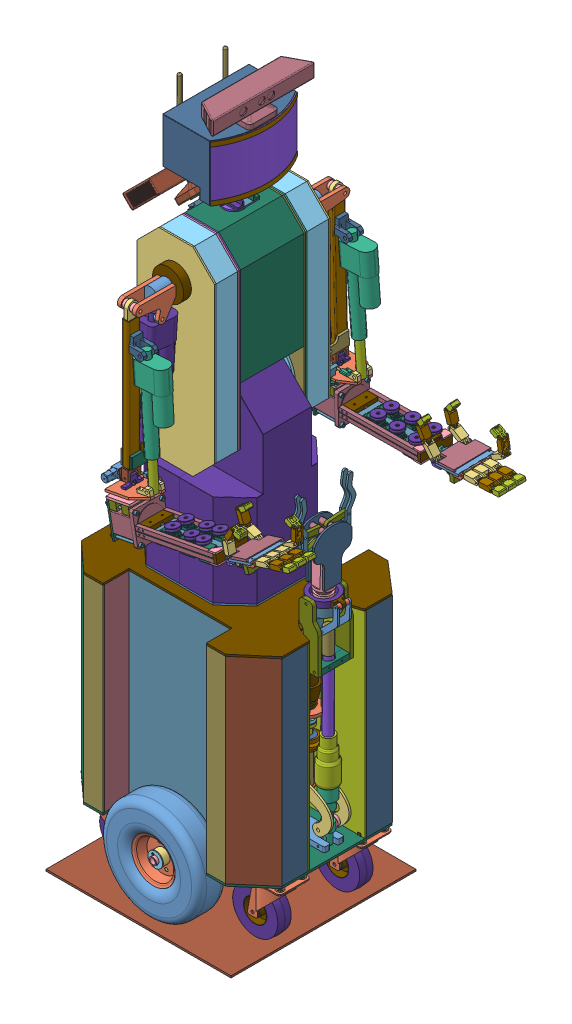
SolidWorks assembly sorbot, configuration По умолчанию. Lengths in mm. (continued)
Components (placement in the parent): (continued)
- bolt1-1: bolt1 [По умолчанию] at (252.2608 28.1179 -56.3731) x (0 0 1) z (1 0 0) size (14 40.5 16.17)
- bolt1-2: bolt1 [По умолчанию] at (172.9115 28.0264 3.3236) x (0 0 1) z (1 0 0) size (14 40.5 16.17)
- bolt1-3: bolt1 [По умолчанию] at (251.9125 28.1164 3.3175) x (0 0 1) z (1 0 0) size (14 40.5 16.17)
- bolt1-4: bolt1 [По умолчанию] at (172.9018 28.0211 -56.2899) x (0 0 1) z (1 0 0) size (14 40.5 16.17)
- bolt1-5: bolt1 [По умолчанию] at (172.7717 28.5111 -218.0055) x (0.546944 0 -0.837169) z (-0.837169 0 -0.546944) size (14 40.5 16.17)
- bolt1-6: bolt1 [По умолчанию] at (251.718 28.5111 -277.7613) x (0.546944 0 -0.837169) z (-0.837169 0 -0.546944) size (14 40.5 16.17)
- bolt1-7: bolt1 [По умолчанию] at (172.7558 28.5111 -277.7529) x (0.546944 0 -0.837169) z (-0.837169 0 -0.546944) size (14 40.5 16.17)
- bolt1-8: bolt1 [По умолчанию] at (251.8056 28.5111 -218.1439) x (0.546944 0 -0.837169) z (-0.837169 0 -0.546944) size (14 40.5 16.17)
- bolt1-9: bolt1 [По умолчанию] at (-260.5376 28.2059 -219.1987) x (0.546944 0 -0.837169) z (-0.837169 0 -0.546944) size (14 40.5 16.17)
- bolt1-10: bolt1 [По умолчанию] at (-181.6432 28.2059 -219.1307) x (0.546944 0 -0.837169) z (-0.837169 0 -0.546944) size (14 40.5 16.17)
- bolt1-11: bolt1 [По умолчанию] at (-181.4767 28.2059 -278.9161) x (0.546944 0 -0.837169) z (-0.837169 0 -0.546944) size (14 40.5 16.17)
- bolt1-12: bolt1 [По умолчанию] at (-260.5141 28.2059 -278.9485) x (0.546944 0 -0.837169) z (-0.837169 0 -0.546944) size (14 40.5 16.17)
- bolt1-13: bolt1 [По умолчанию] at (-260.8842 28.1192 -54.1025) x (-0.546944 0 0.837169) z (0.837169 0 0.546944) size (14 40.5 16.17)
- bolt1-14: bolt1 [По умолчанию] at (-181.8952 28.1192 -54.0898) x (-0.546944 0 0.837169) z (0.837169 0 0.546944) size (14 40.5 16.17)
- bolt1-15: bolt1 [По умолчанию] at (-260.8825 28.1192 5.6198) x (-0.546944 0 0.837169) z (0.837169 0 0.546944) size (14 40.5 16.17)
- bolt1-16: bolt1 [По умолчанию] at (-181.994 28.1192 5.6123) x (-0.546944 0 0.837169) z (0.837169 0 0.546944) size (14 40.5 16.17)
- bolt1.nut-1: bolt1.nut [По умолчанию] at (-181.4767 51.9368 -278.9161) x (0 0 1) z (-1 0 0) size (14 6 16.17)
- bolt1.nut-2: bolt1.nut [По умолчанию] at (-260.5141 51.9368 -278.9485) x (0 0 1) z (-1 0 0) size (14 6 16.17)
- bolt1.nut-3: bolt1.nut [По умолчанию] at (-260.5376 51.9368 -219.1987) x (0 0 1) z (-1 0 0) size (14 6 16.17)
- bolt1.nut-4: bolt1.nut [По умолчанию] at (-181.6432 51.9368 -219.1307) x (0 0 1) z (-1 0 0) size (14 6 16.17)
- bolt1.nut-5: bolt1.nut [По умолчанию] at (-181.994 51.9368 5.6123) x (0 0 -1) z (1 0 0) size (14 6 16.17)
- bolt1.nut-6: bolt1.nut [По умолчанию] at (-260.8825 51.9368 5.6198) x (0 0 -1) z (1 0 0) size (14 6 16.17)
- bolt1.nut-7: bolt1.nut [По умолчанию] at (-260.8842 51.9368 -54.1025) x (0 0 -1) z (1 0 0) size (14 6 16.17)
- bolt1.nut-8: bolt1.nut [По умолчанию] at (-181.8952 51.9368 -54.0898) x (0 0 -1) z (1 0 0) size (14 6 16.17)
- bolt1.nut-9: bolt1.nut [По умолчанию] at (172.9115 51.9368 3.3236) x (0 0 -1) z (1 0 0) size (14 6 16.17)
- bolt1.nut-10: bolt1.nut [По умолчанию] at (251.9125 51.7388 3.3175) x (0 0 -1) z (1 0 0) size (14 6 16.17)
- bolt1.nut-11: bolt1.nut [По умолчанию] at (252.2608 51.5573 -56.3731) x (0 0 -1) z (1 0 0) size (14 6 16.17)
- bolt1.nut-12: bolt1.nut [По умолчанию] at (172.9018 51.3675 -56.2899) x (0 0 -1) z (1 0 0) size (14 6 16.17)
- bolt1.nut-13: bolt1.nut [По умолчанию] at (172.7558 51.9368 -277.7529) x (0 0 1) z (-1 0 0) size (14 6 16.17)
- bolt1.nut-14: bolt1.nut [По умолчанию] at (172.7717 51.9368 -218.0055) x (0 0 1) z (-1 0 0) size (14 6 16.17)
- bolt1.nut-15: bolt1.nut [По умолчанию] at (251.718 51.9368 -277.7613) x (0 0 1) z (-1 0 0) size (14 6 16.17)
- bolt1.nut-16: bolt1.nut [По умолчанию] at (251.8056 51.9368 -218.1439) x (0 0 1) z (-1 0 0) size (14 6 16.17)
- turret.table-1: turret.table [По умолчанию] at (-20.8718 607.7934 -141.039) size (305 5 278)
- turret.center-1: turret.center [По умолчанию] at (-20.0648 607.7934 -136.9555) x (1 0 -0.000338) z (0.000338 0 1) size (90 80 90)
- body.center-1: body.center [По умолчанию] at (-20.0648 627.0246 -136.9555) size (22 355 22)
- wheel.axis.frame.fixture.p1-1: wheel.axis.frame.fixture.p1 [По умолчанию] at (40.6964 23.6368 -47.3934) x (0.999999 0 0.001149) z (-0.001149 0 0.999999) size (21.7 48.8 22.74)
- wheel.axis.frame.fixture.p1-2: wheel.axis.frame.fixture.p1 [По умолчанию] at (-54.5345 23.6368 -47.3503) size (21.7 48.8 22.74)
- wheel.axis.frame.fixture.p1-3: wheel.axis.frame.fixture.p1 [По умолчанию] at (40.6515 23.6368 -224.9519) size (21.7 48.8 22.74)
- wheel.axis.frame.fixture.p1-4: wheel.axis.frame.fixture.p1 [По умолчанию] at (-54.2945 23.6368 -224.8346) size (21.7 48.8 22.74)
- gearmotor.fixture.p2.1-1: gearmotor.fixture.p2.1 [По умолчанию] at (2.1309 53.4368 -208.1692) x (-1 0 0) z (0 0 -1) size (86 101.43 182)
- wheel.axis.frame.fixture.p2-1: wheel.axis.frame.fixture.p2 [По умолчанию] at (40.6964 51.9368 -47.3934) size (22.08 10 22.5)
- wheel.axis.frame.fixture.p2-2: wheel.axis.frame.fixture.p2 [По умолчанию] at (40.6515 53.4933 -224.9519) size (22.08 10 22.5)
- wheel.axis.frame.fixture.p2-3: wheel.axis.frame.fixture.p2 [По умолчанию] at (-54.2945 53.4933 -224.8346) size (22.08 10 22.5)
- wheel.axis.frame.fixture.p2-4: wheel.axis.frame.fixture.p2 [По умолчанию] at (-54.5345 53.4933 -47.3503) size (22.08 10 22.5)
- wall-fixture-3-2: wall-fixture-3 [По умолчанию] at (-150.6756 56.9368 4.4522) size (287.58 65 40)
- wall-fixture-3-1-1: wall-fixture-3-1 [По умолчанию] at (-154.6756 56.9368 4.4522) x (0 0 -1) z (1 0 0) size (74 65 40)
- wall-fixture-3-2-1: wall-fixture-3-2 [По умолчанию] at (-154.6756 56.9368 74.4522) size (42 65 40)
- wall-fixture-3-3-1: wall-fixture-3-3 [По умолчанию] at (-194.4824 56.9368 75.4251) x (0.73854 0 0.67421) z (-0.67421 0 0.73854) size (116.95 65 40)
- ground-1: ground [По умолчанию] at (-17.2598 -128.0632 -134.3184) size (500 5 500)
- body_pivot_fixture-1: body_pivot_fixture [По умолчанию] at (-20.0648 922.0246 -136.9555) x (0.99898 0 -0.04516) z (0.04516 0 0.99898) size (78 60 78)
- body_axis-1: body_axis [По умолчанию] at (-20.0648 1016.5246 -221.0975) x (0.999995 0.003042 0) z (0 0 1) size (21.8 21.8 170.35)
- body_tilt_drive_frame_p1-1: body_tilt_drive_frame_p1 [По умолчанию] at (-111.0648 612.7934 -275.9555) x (0.999999 0 0.001245) z (-0.001245 0 0.999999) size (186.87 100 2.5) (hidden)
- body_tilt_drive_frame_p1-2: body_tilt_drive_frame_p1 [По умолчанию] at (70.9352 612.7934 2.0445) x (-1 0 0) z (0 0 -1) size (186.87 100 2.5) (hidden)
- body_tilt_drive_frame_p2-1: body_tilt_drive_frame_p2 [По умолчанию] at (-169.3526 612.7934 -55.387) x (0.73343 0 0.679765) z (-0.679765 0 0.73343) size (80.39 100 2.5) (hidden)
- body_tilt_drive_frame_p2-2: body_tilt_drive_frame_p2 [По умолчанию] at (-169.9731 712.7934 -220.8616) x (0.72933 0 -0.684163) z (-0.684163 0 -0.72933) size (80.39 100 2.5) (hidden)
- body_tilt_drive_frame_p3-1: body_tilt_drive_frame_p3 [По умолчанию] at (-173.1373 612.7934 -144.4799) x (0 0 -1) z (1 0 0) size (167.12 100 2.5) (hidden)
- body_tilt_drive_frame_p4-1: body_tilt_drive_frame_p4 [По умолчанию] at (130.9977 612.7934 -221.3211) x (0 0 1) z (-1 0 0) size (167.12 100 2.5) (hidden)
- body_tilt_drive_frame_p5-1: body_tilt_drive_frame_p5 [По умолчанию] at (65.0237 612.7934 -7.7276) x (0.72933 0 -0.684163) z (0.684163 0 0.72933) size (80.39 100 2.5) (hidden)
- body_tilt_drive_frame_p5-2: body_tilt_drive_frame_p5 [По умолчанию] at (78.6946 612.7934 -282.3701) x (0.72933 0 0.684163) z (-0.684163 0 0.72933) size (80.39 100 2.5) (hidden)
- turret.table.cap-1: turret.table.cap [По умолчанию] at (-20.0648 712.7934 -136.9555) size (304.13 2.5 277.12) (hidden)
- body_tilt_drive_frame_p6-2: body_tilt_drive_frame_p6 [По умолчанию] at (-175.1373 715.2934 -67.4448) x (1 0 0) z (0 0 1) size (300.14 367.75 2.5) (hidden)
- body_tilt_drive_frame_cap-1: body_tilt_drive_frame_cap [По умолчанию] at (-171.1373 715.2934 -64.9448) x (1 0 0) z (0 0 1) size (304.13 369.75 142) (hidden)
- body_tilt_drive_frame_p6-3: body_tilt_drive_frame_p6 [По умолчанию] at (-175.1373 715.2934 -206.9448) x (1 0 0) z (0 0 1) size (300.14 367.75 2.5) (hidden)
- body.frame.p1.fixture-1: body.frame.p1.fixture [По умолчанию] at (-20.8083 1016.2071 -56.7442) x (-0.989237 -0.146324 0) z (0 0 -1) size (89 89 22)
- body.frame.p1.fixture-2: body.frame.p1.fixture [По умолчанию] at (-20.0648 1016.5246 -216.3595) x (0.862438 0.506162 0) z (0 0 1) size (89 89 22)
- body.frame.p2-1: body.frame.p2 [По умолчанию] at (-4.2156 797.7971 -50.7442) x (-1 0 0) z (0 0 -1) size (210 323.57 171.62)
- body.frame.p3-1: body.frame.p3 [По умолчанию] at (94.3623 1112.7235 -40.8506) x (-1 0 0) z (0 0 -1) size (206 2 171.62)
- arm.actuator-1: arm.actuator [Default] at (-100.027 1094.2768 -11.7544) x (0 0 -1) z (0.997693 -0.067885 0) size (42 292 82)
  - arm.actuator.p1-1: arm.actuator.p1 [Default] at (1.9897 -28.1276 18.0595) size (42 292 82)
- arm.actuator.p2-1: arm.actuator.p2 [Default] at (-71.299 1250.4551 -13.7442) x (-0.997693 0.067885 0) z (0 0 -1) size (20 180 20)
- arm.lift.actuator.fixture.p2-1: arm.lift.actuator.fixture.p2 [По умолчанию] at (-88.5767 993.1387 -41.8307) x (0.99962 0.027553 0) z (0 0 1) size (8 8 57)
- shoulder.p4-1: shoulder.p4 [По умолчанию] at (-12.6529 1335.4871 -25.7442) x (0.590367 -0.807135 0) z (0 0 1) size (124.11 60 4)
- shoulder.p4-2: shoulder.p4 [По умолчанию] at (-12.6483 1335.4904 -1.7442) x (0.590423 -0.807094 0) z (0 0 1) size (124.11 60 4)
- arm.lift.actuator.fixture.p3-1: arm.lift.actuator.fixture.p3 [По умолчанию] at (-88.5767 993.1387 15.2558) x (-1 -0.000227 0) z (0 0 -1) size (39.1 39.1 19)
- arm.lift.actuator.fixture.p3-2: arm.lift.actuator.fixture.p3 [По умолчанию] at (-88.5767 993.1387 -42.7442) x (1 -0.000113 0) z (0 0 1) size (39.1 39.1 19)
- shoulder.p6-1: shoulder.p6 [По умолчанию] at (-12.6457 1335.4135 -42.7442) x (-0.13701 -0.99057 0) z (0 0 1) size (53.6 53.6 22)
- shoulder.p6-2: shoulder.p6 [По умолчанию] at (-12.6483 1335.4904 16.6679) x (-0.526603 0.850111 0) z (0 0 -1) size (53.6 53.6 22)
- body.frame.p5-1: body.frame.p5 [По умолчанию] at (-12.763 795.3888 -42.7442) x (1 0 0) z (0 0 1) size (210 537.69 58)
- arm.actuator-2: arm.actuator [Default] at (-14.7745 1188.0283 105.1323) x (1 0 0) z (0 -0.068351 -0.997661) size (42 292 82)
  - arm.actuator.p1-1: arm.actuator.p1 [Default] at (1.9897 -28.1276 18.0595) size (42 292 82)
- arm.actuator.p2-2: arm.actuator.p2 [Default] at (-12.7848 1126.9341 91.2161) x (0 -0.068351 -0.997661) z (-1 0 0) size (20 180 20)
- arm.actuator100mm..p1-1: arm.actuator100mm..p1 [Default] at (34.2144 1176.4747 140.2746) x (0 0 1) z (0.998134 0.061067 0) size (42 244 82)
- arm.actuator100mm.p2-1: arm.actuator100mm.p2 [Default] at (41.3177 1060.3732 140.2746) x (0.998134 0.061067 0) z (0 0 -1) size (20 130 20)
- body.frame.p1-3: body.frame.p1 [По умолчанию] at (-12.5732 795.4676 -50.7442) x (1 0 0) z (0 0 1) size (210 537.56 4)
- cap-hinge-1: cap-hinge [По умолчанию] at (95.4017 1285.4557 -46.5922) x (0 0 1) z (0 1 0) size (35.83 6 40) (hidden)
- cap-hinge-p1-1: cap-hinge-p1 [По умолчанию] at (95.4017 1326.2182 -46.5922) x (0 0 -1) z (0 -1 0) size (35.83 6 40) (hidden)
- cap-hinge-2: cap-hinge [По умолчанию] at (95.4017 1183.4534 -46.8053) x (0 0 -1) z (0 -1 0) size (35.83 6 40) (hidden)
- cap-hinge-p1-2: cap-hinge-p1 [По умолчанию] at (95.4017 1142.6154 -46.8053) x (0 0 1) z (0 1 0) size (35.83 6 40) (hidden)
- arm.p1.m-1: arm.p1.m [По умолчанию] at (-12.763 1309.7884 140.1602) x (1 0 0) z (0 0 -1) size (18 345 32.5)
- actuator.100.fixture-1: actuator.100.fixture [По умолчанию] at (23.3566 1237.5198 140.1602) x (0 0 1) z (-1 0 0) size (40 40 44)
- forearm.rotate.p9-1: forearm.rotate.p9 [По умолчанию] at (-4.2763 976.7014 103.5825) x (-1 0 0) z (0 0 1) size (18 63 34)
- forearm.rotate.p12-1: forearm.rotate.p12 [По умолчанию] at (-21.7679 963.9 61.4944) x (1 0 0) z (0 0 -1) size (7 35 61.58)
- lower.arm.p2-1: lower.arm.p2 [По умолчанию] at (41.5663 863.9612 178.2746) x (0.982605 0.185706 0) z (0 0 1) size (214 10 10)
- lower.arm.p2-2: lower.arm.p2 [По умолчанию] at (43.7948 852.17 178.2746) x (0.982605 0.185706 0) z (0 0 -1) size (214 10 10)
- lower.arm.p2-3: lower.arm.p2 [По умолчанию] at (41.5663 863.9612 102.2746) x (0.982605 0.185706 0) z (0 0 1) size (214 10 10)
- lower.arm.p2-4: lower.arm.p2 [По умолчанию] at (43.7948 852.17 102.2746) x (0.982605 0.185706 0) z (0 0 -1) size (214 10 10)
- lower.arm.p3-1: lower.arm.p3 [По умолчанию] at (41.8837 856.8973 100.2593) x (0.982605 0.185706 0) z (0 0 1) size (214 2 86)
- HS-311 Hitec Standard Servo and Horn-1: HS-311 Hitec Standard Servo and Horn [Default] at (126.5902 849.0921 157.9974) x (0 0 1) z (-0.982605 -0.185706 0) size (27.94 44.98 53.29)
  - HS-311 Hitec Standard Servo-1: HS-311 Hitec Standard Servo [Default] at origin size (20.32 41.27 53.29)
  - HS-311-p2-1: HS-311-p2 [По умолчанию] at (0 42.485 0) x (0.967717 0 0.252038) z (-0.252038 0 0.967717) size (22.63 6.25 24)
- HS-311 Hitec Standard Servo and Horn-2: HS-311 Hitec Standard Servo and Horn [Default] at (180.6335 859.3059 119.9974) x (0 0 1) z (-0.982605 -0.185706 0) size (27.94 44.98 53.29)
  - HS-311 Hitec Standard Servo-1: HS-311 Hitec Standard Servo [Default] at origin size (20.32 41.27 53.29)
  - HS-311-p2-1: HS-311-p2 [По умолчанию] at (0 42.485 0) x (0.967717 0 0.252038) z (-0.252038 0 0.967717) size (22.63 6.25 24)
- HS-311 Hitec Standard Servo and Horn-3: HS-311 Hitec Standard Servo and Horn [Default] at (126.5902 849.0921 122.4974) x (0 0 1) z (-0.982605 -0.185706 0) size (27.94 44.98 53.29)
  - HS-311 Hitec Standard Servo-1: HS-311 Hitec Standard Servo [Default] at origin size (20.32 41.27 53.29)
  - HS-311-p2-1: HS-311-p2 [По умолчанию] at (0 42.485 0) x (0.967717 0 0.252038) z (-0.252038 0 0.967717) size (22.63 6.25 24)
- HS-311 Hitec Standard Servo and Horn-4: HS-311 Hitec Standard Servo and Horn [Default] at (214.3565 865.6794 117.4346) x (0 0 -1) z (0.982605 0.185706 0) size (27.94 44.98 53.29)
  - HS-311 Hitec Standard Servo-1: HS-311 Hitec Standard Servo [Default] at origin size (20.32 41.27 53.29)
  - HS-311-p2-1: HS-311-p2 [По умолчанию] at (0 42.485 0) x (0.967717 0 0.252038) z (-0.252038 0 0.967717) size (22.63 6.25 24)
- HS-311 Hitec Standard Servo and Horn-5: HS-311 Hitec Standard Servo and Horn [Default] at (180.6335 859.3059 160.9974) x (0 0 1) z (-0.982605 -0.185706 0) size (27.94 44.98 53.29)
  - HS-311 Hitec Standard Servo-1: HS-311 Hitec Standard Servo [Default] at origin size (20.32 41.27 53.29)
  - HS-311-p2-1: HS-311-p2 [По умолчанию] at (0 42.485 0) x (0.967717 0 0.252038) z (-0.252038 0 0.967717) size (22.63 6.25 24)
- HS-311 Hitec Standard Servo and Horn-6: HS-311 Hitec Standard Servo and Horn [Default] at (214.3565 865.6794 163.1146) x (0 0 -1) z (0.982605 0.185706 0) size (27.94 44.98 53.29)
  - HS-311 Hitec Standard Servo-1: HS-311 Hitec Standard Servo [Default] at origin size (20.32 41.27 53.29)
  - HS-311-p2-1: HS-311-p2 [По умолчанию] at (0 42.485 0) x (0.967717 0 0.252038) z (-0.252038 0 0.967717) size (22.63 6.25 24)
- lower.arm.p9-1: lower.arm.p9 [По умолчанию] at (119.1648 888.3816 157.9974) x (0.982605 0.185706 0) z (0 0 1) size (32.15 8 32.15)
- lower.arm.p9-2: lower.arm.p9 [По умолчанию] at (119.1648 888.3816 122.4974) x (0.982605 0.185706 0) z (0 0 1) size (32.15 8 32.15)
- lower.arm.p9-3: lower.arm.p9 [По умолчанию] at (206.9311 904.9689 163.1146) x (-0.982605 -0.185706 0) z (0 0 -1) size (32.15 8 32.15)
- lower.arm.p9-4: lower.arm.p9 [По умолчанию] at (173.2081 898.5954 160.9974) x (0.982605 0.185706 0) z (0 0 1) size (32.15 8 32.15)
- lower.arm.p9-5: lower.arm.p9 [По умолчанию] at (173.2081 898.5954 119.9974) x (0.982605 0.185706 0) z (0 0 1) size (32.15 8 32.15)
- lower.arm.p9-6: lower.arm.p9 [По умолчанию] at (206.9311 904.9689 117.4346) x (-0.982605 -0.185706 0) z (0 0 -1) size (32.15 8 32.15)
- lower.arm.p8-2: lower.arm.p8 [По умолчанию] at (250.9153 908.6154 183.2746) x (0.982605 0.185706 0) z (0 0 1) size (8 36.31 86)
- palm.p1-3: palm.p1 [По умолчанию] at (326.2301 928.273 153.074) x (0.950144 0.311545 0.012888) z (-0.012247 -0.004016 0.999917) size (75 6 100)
- palm.p3-1: palm.p3 [По умолчанию] at (374.5143 939.8955 115.7089) x (-0.012247 -0.004016 0.999917) z (-0.950144 -0.311545 -0.012888) size (100 13.5 26)
- finger.p1-1: finger.p1 [По умолчанию] at (361.4218 946.6526 179.831) x (0.950144 0.311545 0.012888) z (-0.012247 -0.004016 0.999917) size (50 12 20.5)
- palm.fixture.p4-1: palm.fixture.p4 [По умолчанию] at (258.7762 910.1011 183.2746) x (0 0 -1) z (0.982605 0.185706 0) size (25 4 20)
- palm.fixture.p4-3: palm.fixture.p4 [По умолчанию] at (263.6045 884.5534 183.2746) x (0 0 -1) z (0.982605 0.185706 0) size (25 4 20)
- palm.fixture.p4-4: palm.fixture.p4 [По умолчанию] at (258.7762 910.1011 97.2746) x (-0.982605 -0.185706 0) z (0 0 -1) size (25 4 20)
- palm.fixture.p4-5: palm.fixture.p4 [По умолчанию] at (262.8617 888.4838 97.2746) x (0 0 1) z (0.982605 0.185706 0) size (25 4 20)
- finger.spring-1: finger.spring [По умолчанию] at (366.5011 947.2657 178.5056) x (0.311571 -0.950223 0) z (-0.012247 -0.004016 0.999917) size (5.38 21 4.23)
- palm.fixture.p13-1: palm.fixture.p13 [По умолчанию] at (366.3409 947.2132 191.5879) x (0.430913 -0.902392 0.001654) z (0.012247 0.004016 -0.999917) size (3 3 100)
- finger.spring-2: finger.spring [По умолчанию] at (405.9116 957.8496 176.7806) x (0.327007 -0.945022 0.00021) z (-0.012247 -0.004016 0.999917) size (5.38 21 4.23)
- finger.p3-1: finger.p3 [По умолчанию] at (437.7359 970.6062 180.9748) x (0.950144 0.311546 0.012888) z (-0.012247 -0.004016 0.999917) size (30 12 20.5)
- finger.p1-2: finger.p1 [По умолчанию] at (362.6718 945.7123 103.3362) x (0.841955 0.539404 0.012478) z (-0.012247 -0.004016 0.999917) size (50 12 20.5)
- finger.p3-2: finger.p3 [По умолчанию] at (404.7341 1004.7181 104.2012) x (-0.905154 0.424979 -0.00938) z (-0.012247 -0.004016 0.999917) size (30 12 20.5)
- finger.p1-3: finger.p1 [По умолчанию] at (361.7341 946.755 154.3331) x (0.950144 0.311545 0.012888) z (-0.012247 -0.004016 0.999917) size (50 12 20.5)
- finger.p3-3: finger.p3 [По умолчанию] at (437.7976 971.5136 155.4898) x (0.950144 0.311546 0.012888) z (-0.012247 -0.004016 0.999917) size (30 12 20.5)
- palm.p3.m-1: palm.p3.m [По умолчанию] at (294.6906 913.722 190.6324) x (0.012247 0.004016 -0.999917) z (0.950144 0.311545 0.012888) size (21.5 12 26)
- finger.p1-4: finger.p1 [По умолчанию] at (362.0464 946.8574 128.8352) x (0.950144 0.311545 0.012888) z (-0.012247 -0.004016 0.999917) size (50 12 20.5)
- finger.p3-4: finger.p3 [По умолчанию] at (438.0521 971.8022 129.7881) x (0.950144 0.311546 0.012888) z (-0.012247 -0.004016 0.999917) size (30 12 20.5)
- palm.p3.m-2: palm.p3.m [По умолчанию] at (295.652 914.0372 112.1389) x (0.012247 0.004016 -0.999917) z (0.950144 0.311545 0.012888) size (21.5 12 26)
- finger.p1-5: finger.p1 [По умолчанию] at (298.6941 917.8741 179.9472) x (-0.206644 0.978415 0.001398) z (0.012247 0.004016 -0.999917) size (50 12 20.5)
- finger.p3-5: finger.p3 [По умолчанию] at (303.3786 994.7192 180.4261) x (0.98461 -0.174397 0.011359) z (0.012247 0.004016 -0.999917) size (30 12 20.5)
- finger.p1-6: finger.p1 [По умолчанию] at (302.6817 922.0965 101.6065) x (-0.939132 0.343406 -0.010123) z (0.012247 0.004016 -0.999917) size (50 12 20.5)
- finger.p3-6: finger.p3 [По умолчанию] at (242.2623 968.6455 101.1663) x (0.802448 0.596597 0.012224) z (0.012247 0.004016 -0.999917) size (30 12 20.5)
- finger.p2-7: finger.p2 [По умолчанию] at (400.3799 959.5495 180.36) x (0.957938 0.286686 0.012884) z (-0.012247 -0.004016 0.999917) size (48 12 20.5)
- finger.p2-8: finger.p2 [По умолчанию] at (400.6902 959.5494 154.8616) x (0.951517 0.307327 0.012888) z (-0.012247 -0.004016 0.999917) size (48 12 20.5)
- finger.p2-9: finger.p2 [По умолчанию] at (401.0023 959.6281 129.3637) x (0.949969 0.312079 0.012888) z (-0.012247 -0.004016 0.999917) size (48 12 20.5)
- finger.p2-10: finger.p2 [По умолчанию] at (400.3467 964.4738 103.873) x (-0.01257 0.999914 0.003862) z (-0.012247 -0.004016 0.999917) size (48 12 20.5)
- finger.p2-11: finger.p2 [По умолчанию] at (286.7699 957.4574 179.9601) x (0.519178 0.85461 0.009791) z (0.012247 0.004016 -0.999917) size (48 12 20.5)
- finger.p2-12: finger.p2 [По умолчанию] at (262.4973 932.6893 101.1569) x (-0.370677 0.928761 -0.00081) z (0.012247 0.004016 -0.999917) size (48 12 20.5)
- finger1.rod-1: finger1.rod [По умолчанию] at (453.9909 979.577 179.5221) x (0.950144 0.311546 0.012888) z (-0.012247 -0.004016 0.999917) size (196.04 3.19 32.22)
- palm.p5-1: palm.p5 [По умолчанию] at (330.6828 936.0474 170.4076) x (0.950144 0.311545 0.012888) z (-0.012247 -0.004016 0.999917) size (21.8 4 21.8)
- palm.p6-1: palm.p6 [По умолчанию] at (301.0674 926.3367 156.6492) x (0.950144 0.311545 0.012888) z (-0.012247 -0.004016 0.999917) size (13.8 4 13.8)
- palm.p5-2: palm.p5 [По умолчанию] at (331.3758 936.2746 112.4456) x (0.950144 0.311545 0.012888) z (-0.012247 -0.004016 0.999917) size (21.8 4 21.8)
- palm.p6-2: palm.p6 [По умолчанию] at (301.386 926.4412 124.555) x (0.950144 0.311545 0.012888) z (-0.012247 -0.004016 0.999917) size (13.8 4 13.8)
- palm.cap-1: palm.cap [По умолчанию] at (361.9011 946.2836 191.5864) x (0.950144 0.311545 0.012888) z (-0.012247 -0.004016 0.999917) size (62.89 6 100)
- palm.fixture.p14-1: palm.fixture.p14 [По умолчанию] at (275.8203 911.7441 155.3904) x (0.950144 0.311545 0.012888) z (-0.012247 -0.004016 0.999917) size (45 6 30)
- forearm.rotate.p12-m-1: forearm.rotate.p12-m [По умолчанию] at (3.237 963.9 61.4944) x (1 0 0) z (0 0 -1) size (7 30.01 61.58)
- arm.fixture.cap-1: arm.fixture.cap [По умолчанию] at (-12.4559 1335.4922 -51.2442) x (0.999995 -0.003183 0) z (0.003183 0.999995 0) size (110 23 110)
- body_tilit_stud-1: body_tilit_stud [По умолчанию] at (-48.2188 648.7352 -136.446) x (1 0 -0.000338) z (0.000338 0 1) size (6 307 6)
- shoulder.bearing.housing-1: shoulder.bearing.housing [По умолчанию] at (-12.7629 1335.3853 19.2558) x (1 0 0) z (0 0 1) size (84 84 21)
- shoulder.bearing.housing-2: shoulder.bearing.housing [По умолчанию] at (-12.4903 1335.516 -46.7442) x (-0.799769 0.600308 0) z (0 0 -1) size (84 84 21)
- shoulder.axis-1: shoulder.axis [По умолчанию] at (-12.7629 1335.3853 -67.7442) x (1 0 0) z (0 0 1) size (30 40 157)
- arm.fixture-2: arm.fixture [По умолчанию] at (-27.7629 1348.6141 44.2558) x (-1 0 0) z (0 0 -1) size (10 73.07 108.23)
- shoulder.lever-1: shoulder.lever [По умолчанию] at (-7.763 1350.5713 104.4102) x (-1 0 0) z (0 0 -1) size (10 77.8 28.5)
- arm.lift2.actuator.fixture.p1-1: arm.lift2.actuator.fixture.p1 [По умолчанию] at (-27.763 1335.3853 140.1602) x (1 0 0) z (0 -0.000978 1) size (10 20 20)
- arm.lift2.actuator.fixture.p1.m1-1: arm.lift2.actuator.fixture.p1.m1 [По умолчанию] at (-27.7629 1286.6873 80.2712) x (1 0 0) z (0 -0.000962 1) size (5 20 20)
- arm.fixture-3: arm.fixture [По умолчанию] at (12.2371 1348.614 44.2558) x (-1 0 0) z (0 0 -1) size (10 73.07 108.23)
- arm.lift2.actuator.fixture.p1-3: arm.lift2.actuator.fixture.p1 [По умолчанию] at (-7.7629 1335.3853 140.1602) x (1 0 0) z (0 -0.000978 1) size (10 20 20)
- arm.lift2.actuator.fixture.p1.m1-2: arm.lift2.actuator.fixture.p1.m1 [По умолчанию] at (-2.7629 1286.6873 80.2712) x (1 0 0) z (0 -0.000962 1) size (5 20 20)
- body_pivot-2: body_pivot [По умолчанию] at (-55.8885 972.0246 -153.8981) x (1 0 0) z (0 0 1) size (140 10 130)
- body.tilt.axis.frame-2: body.tilt.axis.frame [По умолчанию] at (29.9352 1018.0246 -79.5942) x (-1 0 0) z (0 0 -1) size (126 65.5 38)
- body.tilt.axis.frame-3: body.tilt.axis.frame [По умолчанию] at (-70.0648 1018.0246 -194.4875) x (1 0 0) z (0 0 1) size (126 65.5 38)
- tilt.thread.rod-1: tilt.thread.rod [По умолчанию] at (-119.3768 729.5591 -141.6211) x (0.714335 0 -0.699804) z (0.699804 0 0.714335) size (16 154 16)
- tilt.thread.rod.fixture.2-1: tilt.thread.rod.fixture.2 [По умолчанию] at (-119.3768 793.5591 -141.6211) size (40 26 40)
- tilit.thread.rod.bearing.fixture-1: tilit.thread.rod.bearing.fixture [По умолчанию] at (-130.6447 929.0246 -154.0466) x (0.999985 0 0.005494) z (-0.005494 0 0.999985) size (171.17 8 70)
- tilit.thread.bearing-1: tilit.thread.bearing [По умолчанию] at (-119.3768 937.0246 -141.6211) size (28 8 28)
- tilit.thread.rod.bearing.housing-1: tilit.thread.rod.bearing.housing [По умолчанию] at (-119.3768 937.0246 -141.6211) size (42.5 10 42.5)
- body_tilt_axis_clamp-1: body_tilt_axis_clamp [По умолчанию] at (-20.0648 1016.5246 -90.4875) x (-0.92275 -0.3854 0) z (0 0 -1) size (65 65 23)
- body_tilt_axis_clamp-2: body_tilt_axis_clamp [По умолчанию] at (-20.0648 1016.5246 -183.5942) x (0.999995 0.003042 0) z (0 0 1) size (65 65 23)
- body_tilt_lever-1: body_tilt_lever [По умолчанию] at (-20.0648 1016.5246 -155.4875) x (0.894303 0.447461 0) z (0 0 1) size (137.08 65 6)
- body_tilt_lever-2: body_tilt_lever [По умолчанию] at (-20.0648 1016.5246 -124.5942) x (0.894303 0.447461 0) z (0 0 1) size (137.08 65 6)
- body.tilit.lever.2-1: body.tilit.lever.2 [По умолчанию] at (-119.3768 828.3995 -181.4655) x (0.133707 0.991021 0) z (-0.991021 0.133707 0) size (179.8 7 30)
- body_tilt_lever_axis-1: body_tilt_lever_axis [По умолчанию] at (-99.3474 976.856 -195.4875) x (-0.131453 -0.991322 0) z (0 0 1) size (10 10 115)
- body.tilt.nut-1: body.tilt.nut [По умолчанию] at (-119.3768 828.3995 -141.6211) x (1 0 -0.000625) z (0.000625 0 1) size (36 14 31.19)
- body.tilit.nut.housing-1: body.tilit.nut.housing [По умолчанию] at (-119.3768 818.3995 -141.6211) x (0 0 -1) z (1 0 0) size (79.69 20 43.97)
- body.tilit.nut.housing.bolt-1: body.tilit.nut.housing.bolt [По умолчанию] at (-119.3768 828.3995 -188.4655) x (0 0 1) z (-1 0 0) size (38 19.4 20.53)
- body.tilit.nut.housing.cap-1: body.tilit.nut.housing.cap [По умолчанию] at (-97.3898 838.3995 -181.4655) x (0 0 1) z (-1 0 0) size (79.69 10 43.97)
- body.tilit.extender-1: body.tilit.extender [По умолчанию] at (-99.3474 976.856 -155.4875) x (0 0 -1) z (1 0 0) size (21.5 30 30)
- washer-1: washer [По умолчанию] at (-99.3474 976.856 -190.4655) x (1 0 0) z (0 0 1) size (24 24 2)
- body.tilit.extender-2: body.tilit.extender [По умолчанию] at (-99.3474 976.856 -97.0942) x (0 0 -1) z (1 0 0) size (21.5 30 30)
- body.tilit.lever.2-2: body.tilit.lever.2 [По умолчанию] at (-119.3768 828.3995 -94.7768) x (0.133707 0.991021 0) z (-0.991021 0.133707 0) size (179.8 7 30)
- body.tilit.nut.housing.bolt-2: body.tilit.nut.housing.bolt [По умолчанию] at (-119.3768 828.3995 -94.7768) x (0 0 -1) z (1 0 0) size (38 19.4 20.53)
- washer-2: washer [По умолчанию] at (-99.3474 976.856 -94.7768) x (1 0 0) z (0 0 1) size (24 24 2)
- body.tilit.enforcement-1: body.tilit.enforcement [По умолчанию] at (-20.8083 1016.2071 -56.7442) x (0.999986 -0.005204 0) z (-0.005204 -0.999986 0) size (178 6 178)
- body.tilit.enforcement-2: body.tilit.enforcement [По умолчанию] at (-20.0648 1016.5246 -222.3595) x (1 0 0) z (0 -1 0) size (178 6 178)
- arm.fixture.cap-2: arm.fixture.cap [По умолчанию] at (-15.2428 1335.4923 -221.8595) x (0.999986 -0.005204 0) z (-0.005204 -0.999986 0) size (110 23 110)
- body.frame.p4-4: body.frame.p4 [По умолчанию] at (-12.3773 795.5195 -230.3595) x (1 0 0) z (0 0 1) size (210 537.56 4)
- body.frame.p5-2: body.frame.p5 [По умолчанию] at (-12.6499 795.3889 -288.3595) x (1 0 0) z (0 0 1) size (210 537.69 58)
- cap-hinge-p1-3: cap-hinge-p1 [По умолчанию] at (95.5097 1287.1115 -226.3787) x (0 0 1) z (0 1 0) size (35.83 6 40) (hidden)
- cap-hinge-4: cap-hinge [По умолчанию] at (95.5097 1143.1735 -226.3787) x (0 0 1) z (0 1 0) size (35.83 6 40) (hidden)
- cap-hinge-5: cap-hinge [По умолчанию] at (95.5097 1327.9494 -226.3787) x (-0.005204 0 -0.999986) z (0 -1 0) size (35.83 6 40) (hidden)
- cap-hinge-p1-4: cap-hinge-p1 [По умолчанию] at (95.5097 1183.936 -226.3787) x (-0.005211 0 -0.999986) z (0 -1 0) size (35.83 6 40) (hidden)
- shoulder.bearing.housing-3: shoulder.bearing.housing [По умолчанию] at (-12.6499 1335.3853 -292.3595) x (1 -0.000001 0) z (0 0 -1) size (84 84 21)
- shoulder.bearing.housing-4: shoulder.bearing.housing [По умолчанию] at (-12.3772 1335.516 -226.3595) x (1 0 0) z (0 0 1) size (84 84 21)
- shoulder.axis-2: shoulder.axis [По умолчанию] at (-12.6499 1335.3853 -205.3595) x (1 0 0) z (0 0 -1) size (30 40 157)
- shoulder.p6-3: shoulder.p6 [По умолчанию] at (-12.6499 1335.3853 -227.2739) x (-0.950595 -0.310432 0) z (0 0 -1) size (53.6 53.6 22)
- shoulder.p6-4: shoulder.p6 [По умолчанию] at (-12.6499 1335.3853 -288.3595) x (1 0 0) z (0 0 1) size (53.6 53.6 22)
- shoulder.p4-3: shoulder.p4 [По умолчанию] at (-12.6499 1335.3853 -247.3595) x (0.588806 -0.808274 0) z (0 0 1) size (124.11 60 4)
- shoulder.p4-4: shoulder.p4 [По умолчанию] at (-12.6499 1335.3853 -268.3595) x (0.588806 -0.808274 0) z (0 0 1) size (124.11 60 4)
- arm.lift.actuator.fixture.p3-3: arm.lift.actuator.fixture.p3 [По умолчанию] at (-88.5702 993.1387 -230.3595) x (-0.619572 -0.78494 0) z (0 0 -1) size (39.1 39.1 19)
- arm.lift.actuator.fixture.p3-4: arm.lift.actuator.fixture.p3 [По умолчанию] at (-88.5702 993.1387 -288.3595) x (0.977487 0.210996 0) z (0 0 1) size (39.1 39.1 19)
- arm.lift.actuator.fixture.p2-2: arm.lift.actuator.fixture.p2 [По умолчанию] at (-88.5702 993.1387 -287.3595) x (0.873274 0.487229 0) z (0 0 1) size (8 8 57)
- arm.actuator-4: arm.actuator [Default] at (-99.8169 1094.2584 -257.3698) x (0 0 -1) z (0.997711 -0.067628 0) size (42 292 82)
  - arm.actuator.p1-1: arm.actuator.p1 [Default] at (1.9897 -28.1276 18.0595) size (42 292 82)
- arm.actuator.p2-4: arm.actuator.p2 [Default] at (-71.1292 1250.4441 -259.3595) x (0.997711 -0.067628 0) z (0 0 1) size (20 180 20)
- arm.fixture-4: arm.fixture [По умолчанию] at (2.3501 1348.6141 -317.3595) x (0.999986 0 0.005196) z (-0.005196 -0.000016 0.999986) size (10 73.07 108.23)
- arm.fixture-5: arm.fixture [По умолчанию] at (-37.6497 1348.6141 -317.4115) x (0.999986 0 0.005196) z (-0.005196 -0.000016 0.999986) size (10 73.07 108.23)
- shoulder.lever-2: shoulder.lever [По умолчанию] at (-17.3387 1349.7788 -377.2903) x (0.999986 0 0.005196) z (-0.005195 -0.022106 0.999742) size (10 77.8 28.5)
- arm.lift2.actuator.fixture.p1-4: arm.lift2.actuator.fixture.p1 [По умолчанию] at (-7.1514 1335.3868 -413.3148) x (0.999986 0 0.005196) z (-0.005196 -0.000016 0.999986) size (10 20 20)
- arm.lift2.actuator.fixture.p1-5: arm.lift2.actuator.fixture.p1 [По умолчанию] at (-27.1515 1335.3868 -413.2628) x (0.999986 0 0.005196) z (-0.005196 0 0.999986) size (10 20 20)
- arm.p1.m-2: arm.p1.m [По умолчанию] at (-12.1088 964.8834 -421.5332) x (0.999986 0 0.005196) z (-0.005195 -0.022106 0.999742) size (18 345 32.5)
- arm.actuator-5: arm.actuator [Default] at (-10.3307 1188.6881 -380.7869) x (-0.999986 0 -0.005196) z (-0.005174 -0.093519 0.995604) size (42 292 82)
  - arm.actuator.p1-1: arm.actuator.p1 [Default] at (1.9897 -28.1276 18.0595) size (42 292 82)
- arm.lift2.actuator.fixture.p1.m1-3: arm.lift2.actuator.fixture.p1.m1 [По умолчанию] at (-2.4627 1286.6879 -353.4014) x (0.999986 0 0.005196) z (-0.005196 0 0.999986) size (5 20 20)
- arm.lift2.actuator.fixture.p1.m1-4: arm.lift2.actuator.fixture.p1.m1 [По умолчанию] at (-27.4627 1286.6879 -353.3754) x (0.999986 0 0.005196) z (-0.005196 0 0.999986) size (5 20 20)
- forearm.rotate.p12-m-2: forearm.rotate.p12-m [По умолчанию] at (-28.517 962.2566 -343.0069) x (-0.999986 0 -0.005196) z (-0.005195 -0.022106 0.999742) size (7 30.01 61.58)
- forearm.rotate.p12-2: forearm.rotate.p12 [По умолчанию] at (-3.5174 962.2566 -342.877) x (-0.999986 0 -0.005196) z (-0.005195 -0.022106 0.999742) size (7 35 61.58)
- forearm.rotate.p9-2: forearm.rotate.p9 [По умолчанию] at (-3.6751 977.684 -457.5619) x (-0.999986 0 -0.005196) z (-0.005195 -0.022106 0.999742) size (18 63 34)
- actuator.100.fixture-2: actuator.100.fixture [По умолчанию] at (23.979 1237.6167 -415.315) x (-0.005195 -0.022106 0.999742) z (-0.999986 0 -0.005196) size (40 40 44)
- arm.actuator100mm..p1-2: arm.actuator100mm..p1 [Default] at (34.5587 1176.5672 -416.4955) x (-0.005195 -0.022106 0.999742) z (0.998347 0.057103 0.006451) size (42 244 82)
- arm.actuator100mm.p2-2: arm.actuator100mm.p2 [Default] at (41.821 1049.9101 -419.2584) x (0.998347 0.057103 0.006451) z (0.005195 0.022106 -0.999742) size (20 130 20)
- lower.arm.p2-5: lower.arm.p2 [По умолчанию] at (28.9806 854.5589 -385.1362) x (0.99991 0.012267 0.005467) z (-0.005195 -0.022106 0.999742) size (214 10 10)
- lower.arm.p2-6: lower.arm.p2 [По умолчанию] at (29.1292 842.5627 -385.4007) x (0.99991 0.012267 0.005467) z (-0.005195 -0.022106 0.999742) size (214 10 10)
- lower.arm.p2-7: lower.arm.p2 [По умолчанию] at (29.3754 856.2389 -461.1166) x (0.99991 0.012267 0.005467) z (-0.005195 -0.022106 0.999742) size (214 10 10)
- lower.arm.p2-8: lower.arm.p2 [По умолчанию] at (29.524 844.2428 -461.3811) x (0.99991 0.012267 0.005467) z (-0.005195 -0.022106 0.999742) size (214 10 10)
- lower.arm.p3-2: lower.arm.p3 [По умолчанию] at (28.4727 849.2735 -463.2911) x (0.99991 0.012267 0.005467) z (-0.005195 -0.022106 0.999742) size (214 2 86)
- lower.arm.p8-3: lower.arm.p8 [По умолчанию] at (242.8734 862.0719 -378.8573) x (0.99991 0.012267 0.005467) z (-0.005195 -0.022106 0.999742) size (8 36.31 86)
- HS-311 Hitec Standard Servo and Horn-7: HS-311 Hitec Standard Servo and Horn [Default] at (166.093 826.2367 -402.7745) x (-0.005195 -0.022106 0.999742) z (-0.99991 -0.012267 -0.005467) size (27.94 44.98 53.29)
  - HS-311 Hitec Standard Servo-1: HS-311 Hitec Standard Servo [Default] at origin size (20.32 41.27 53.29)
  - HS-311-p2-1: HS-311-p2 [По умолчанию] at (0 42.485 0) x (0.967717 0 0.252038) z (-0.252038 0 0.967717) size (22.63 6.25 24)
- HS-311 Hitec Standard Servo and Horn-8: HS-311 Hitec Standard Servo and Horn [Default] at (166.3037 827.1333 -443.3241) x (-0.005195 -0.022106 0.999742) z (-0.99991 -0.012267 -0.005467) size (27.94 44.98 53.29)
  - HS-311 Hitec Standard Servo-1: HS-311 Hitec Standard Servo [Default] at origin size (20.32 41.27 53.29)
  - HS-311-p2-1: HS-311-p2 [По умолчанию] at (0 42.485 0) x (0.967717 0 0.252038) z (-0.252038 0 0.967717) size (22.63 6.25 24)
- HS-311 Hitec Standard Servo and Horn-9: HS-311 Hitec Standard Servo and Horn [Default] at (221.0839 826.8549 -399.9145) x (-0.005195 -0.022106 0.999742) z (-0.99991 -0.012267 -0.005467) size (27.94 44.98 53.29)
  - HS-311 Hitec Standard Servo-1: HS-311 Hitec Standard Servo [Default] at origin size (20.32 41.27 53.29)
  - HS-311-p2-1: HS-311-p2 [По умолчанию] at (0 42.485 0) x (0.967717 0 0.252038) z (-0.252038 0 0.967717) size (22.63 6.25 24)
- HS-311 Hitec Standard Servo and Horn-10: HS-311 Hitec Standard Servo and Horn [Default] at (221.3213 827.8647 -445.5827) x (-0.005195 -0.022106 0.999742) z (-0.99991 -0.012267 -0.005467) size (27.94 44.98 53.29)
  - HS-311 Hitec Standard Servo-1: HS-311 Hitec Standard Servo [Default] at origin size (20.32 41.27 53.29)
  - HS-311-p2-1: HS-311-p2 [По умолчанию] at (0 42.485 0) x (0.967717 0 0.252038) z (-0.252038 0 0.967717) size (22.63 6.25 24)
- HS-311 Hitec Standard Servo and Horn-11: HS-311 Hitec Standard Servo and Horn [Default] at (111.1025 825.6202 -405.7146) x (-0.005195 -0.022106 0.999742) z (-0.99991 -0.012267 -0.005467) size (27.94 44.98 53.29)
  - HS-311 Hitec Standard Servo-1: HS-311 Hitec Standard Servo [Default] at origin size (20.32 41.27 53.29)
  - HS-311-p2-1: HS-311-p2 [По умолчанию] at (0 42.485 0) x (0.967717 0 0.252038) z (-0.252038 0 0.967717) size (22.63 6.25 24)
- HS-311 Hitec Standard Servo and Horn-12: HS-311 Hitec Standard Servo and Horn [Default] at (111.2858 826.4002 -440.9855) x (-0.005195 -0.022106 0.999742) z (-0.99991 -0.012267 -0.005467) size (27.94 44.98 53.29)
  - HS-311 Hitec Standard Servo-1: HS-311 Hitec Standard Servo [Default] at origin size (20.32 41.27 53.29)
  - HS-311-p2-1: HS-311-p2 [По умолчанию] at (0 42.485 0) x (0.967717 0 0.252038) z (-0.252038 0 0.967717) size (22.63 6.25 24)
- lower.arm.p9-7: lower.arm.p9 [По умолчанию] at (110.6073 865.5925 -404.8333) x (0.99855 0.01352 -0.052116) z (0.052397 -0.021363 0.998398) size (32.15 8 32.15)
- lower.arm.p9-8: lower.arm.p9 [По умолчанию] at (110.7906 866.3724 -440.1042) x (0.99855 0.01352 -0.052116) z (0.052397 -0.021363 0.998398) size (32.15 8 32.15)
- lower.arm.p9-9: lower.arm.p9 [По умолчанию] at (165.5978 866.2089 -401.8932) x (0.99855 0.01352 -0.052116) z (0.052397 -0.021363 0.998398) size (32.15 8 32.15)
- lower.arm.p9-10: lower.arm.p9 [По умолчанию] at (165.8085 867.1056 -442.4428) x (0.99855 0.01352 -0.052116) z (0.052397 -0.021363 0.998398) size (32.15 8 32.15)
- lower.arm.p9-11: lower.arm.p9 [По умолчанию] at (220.5887 866.8271 -399.0332) x (0.99855 0.01352 -0.052116) z (0.052397 -0.021363 0.998398) size (32.15 8 32.15)
- lower.arm.p9-12: lower.arm.p9 [По умолчанию] at (220.826 867.837 -444.7014) x (0.99855 0.01352 -0.052116) z (0.052397 -0.021363 0.998398) size (32.15 8 32.15)
- palm.fixture.p4-6: palm.fixture.p4 [По умолчанию] at (250.8727 862.1701 -378.8136) x (0.005195 0.022106 -0.999742) z (0.99991 0.012267 0.005467) size (25 4 20)
- palm.fixture.p4-7: palm.fixture.p4 [По умолчанию] at (251.1947 836.1784 -379.3866) x (0.005195 0.022106 -0.999742) z (0.99991 0.012267 0.005467) size (25 4 20)
- palm.fixture.p4-8: palm.fixture.p4 [По умолчанию] at (251.2699 868.0699 -464.7032) x (-0.005195 -0.022106 0.999742) z (0.99991 0.012267 0.005467) size (25 4 20)
- palm.fixture.p4-9: palm.fixture.p4 [По умолчанию] at (251.5919 842.0782 -465.2763) x (-0.005195 -0.022106 0.999742) z (0.99991 0.012267 0.005467) size (25 4 20)
- palm.fixture.p14-2: palm.fixture.p14 [По умолчанию] at (269.4564 861.0224 -406.5181) x (0.998179 0.059975 0.006513) z (-0.005195 -0.022106 0.999742) size (45 6 30)
- palm.p1-4: palm.p1 [По умолчанию] at (322.3917 864.2684 -409.1721) x (0.998179 0.059975 0.006513) z (-0.005195 -0.022106 0.999742) size (75 6 100)
- palm.p6-3: palm.p6 [По умолчанию] at (295.9379 868.6488 -407.401) x (0.998026 0.059682 0.019549) z (-0.018211 -0.022887 0.999572) size (13.8 4 13.8)
- palm.p6-4: palm.p6 [По умолчанию] at (296.3955 869.3003 -436.0217) x (0.998026 0.059682 0.019549) z (-0.018211 -0.022887 0.999572) size (13.8 4 13.8)
- palm.p5-3: palm.p5 [По умолчанию] at (330.0768 870.2924 -388.4794) x (0.998026 0.059682 0.019549) z (-0.018211 -0.022887 0.999572) size (21.8 4 21.8)
- palm.p5-4: palm.p5 [По умолчанию] at (330.5285 871.7398 -453.6282) x (0.998026 0.059682 0.019549) z (-0.018211 -0.022887 0.999572) size (21.8 4 21.8)
- palm.cap-2: palm.cap [По умолчанию] at (361.6475 871.8083 -370.7916) x (0.998179 0.059975 0.006513) z (-0.005195 -0.022106 0.999742) size (62.89 6 100)
- palm.p3.m-3: palm.p3.m [По умолчанию] at (288.4804 857.3964 -371.4904) x (0.005195 0.022106 -0.999742) z (0.998179 0.059975 0.006513) size (21.5 12 26)
- palm.p3.m-4: palm.p3.m [По умолчанию] at (288.8882 859.1317 -449.9702) x (0.005195 0.022106 -0.999742) z (0.998179 0.059975 0.006513) size (21.5 12 26)
- palm.p3-2: palm.p3 [По умолчанию] at (371.7565 864.0564 -446.93) x (-0.005195 -0.022106 0.999742) z (-0.998179 -0.059975 -0.006513) size (100 13.5 26)
- finger.p1-7: finger.p1 [По умолчанию] at (296.4475 862.3561 -382.0921) x (-0.618608 0.785572 0.014156) z (0.005195 0.022106 -0.999742) size (50 12 20.5)
- finger.p2-13: finger.p2 [По умолчанию] at (270.5619 893.9062 -381.529) x (-0.470174 0.882409 0.017069) z (0.005195 0.022106 -0.999742) size (48 12 20.5)
- finger.p3-7: finger.p3 [По умолчанию] at (247.3729 927.0618 -381.0293) x (0.5845 0.811122 0.020973) z (0.005195 0.022106 -0.999742) size (30 12 20.5)
- finger.p1-8: finger.p1 [По умолчанию] at (297.7094 865.5037 -460.5362) x (-0.837201 0.54684 0.007741) z (0.005195 0.022106 -0.999742) size (50 12 20.5)
- finger.p2-14: finger.p2 [По умолчанию] at (261.4158 885.1756 -460.2898) x (-0.260238 0.965337 0.019993) z (0.005195 0.022106 -0.999742) size (48 12 20.5)
- finger.p3-8: finger.p3 [По умолчанию] at (247.2354 922.2478 -459.4309) x (0.584142 0.81138 0.020977) z (0.005195 0.022106 -0.999742) size (30 12 20.5)
- finger.p1-9: finger.p1 [По умолчанию] at (361.3008 872.5443 -382.5301) x (0.998179 0.059975 0.006513) z (-0.005195 -0.022106 0.999742) size (50 12 20.5)
- finger.p2-15: finger.p2 [По умолчанию] at (402.2262 875.0033 -382.2631) x (0.998179 0.059975 0.006513) z (-0.005195 -0.022106 0.999742) size (48 12 20.5)
- finger.p3-9: finger.p3 [По умолчанию] at (441.1545 877.3398 -381.8962) x (0.998179 0.059975 0.006513) z (-0.005195 -0.022106 0.999742) size (30 12 20.5)
- finger.p1-10: finger.p1 [По умолчанию] at (361.4333 873.108 -408.0235) x (0.998179 0.059975 0.006513) z (-0.005195 -0.022106 0.999742) size (50 12 20.5)
- finger.p2-16: finger.p2 [По умолчанию] at (402.3586 875.567 -407.7565) x (0.998179 0.059975 0.006513) z (-0.005195 -0.022106 0.999742) size (48 12 20.5)
- finger.p3-10: finger.p3 [По умолчанию] at (441.287 877.9035 -407.3897) x (0.998179 0.059975 0.006513) z (-0.005195 -0.022106 0.999742) size (30 12 20.5)
- finger.p1-11: finger.p1 [По умолчанию] at (361.5658 873.6717 -433.517) x (0.998179 0.059975 0.006513) z (-0.005195 -0.022106 0.999742) size (50 12 20.5)
- finger.p2-17: finger.p2 [По умолчанию] at (402.4911 876.1307 -433.2499) x (0.998179 0.059975 0.006513) z (-0.005195 -0.022106 0.999742) size (48 12 20.5)
- finger.p3-11: finger.p3 [По умолчанию] at (441.4195 878.4672 -432.8831) x (0.998179 0.059975 0.006513) z (-0.005195 -0.022106 0.999742) size (30 12 20.5)
- finger.p1-12: finger.p1 [По умолчанию] at (362.0023 871.6766 -459.0654) x (0.841263 0.540379 0.01632) z (-0.005195 -0.022106 0.999742) size (50 12 20.5)
- finger.p2-18: finger.p2 [По умолчанию] at (400.262 890.3329 -458.454) x (-0.145622 0.989115 0.021115) z (-0.005195 -0.022106 0.999742) size (48 12 20.5)
- finger.p3-12: finger.p3 [По умолчанию] at (398.5933 930.0583 -457.4714) x (-0.870974 0.491289 0.006338) z (-0.005195 -0.022106 0.999742) size (30 12 20.5)
- bodu.tilit.axis.enforcement-1: bodu.tilit.axis.enforcement [По умолчанию] at (-20.0648 1016.5246 -221.0975) x (1 0 0) z (0 0 1) size (18 18 170.35)
- body_tilit_stud-5: body_tilit_stud [По умолчанию] at (-33.7006 648.7352 -112.3187) x (0.499707 0 -0.866195) z (0.866195 0 0.499707) size (6 307 6)
- body_tilit_stud-6: body_tilit_stud [По умолчанию] at (-5.5466 648.7352 -112.8281) x (-0.500293 0 -0.865856) z (0.865856 0 -0.500293) size (6 307 6)
- body_tilit_stud-7: body_tilit_stud [По умолчанию] at (8.0892 648.7352 -137.4649) x (-1 0 0.000338) z (-0.000338 0 -1) size (6 307 6)
- body_tilit_stud-8: body_tilit_stud [По умолчанию] at (-6.429 648.7352 -161.5923) x (-0.499707 0 0.866195) z (-0.866195 0 -0.499707) size (6 307 6)
- body_tilit_stud-9: body_tilit_stud [По умолчанию] at (-34.583 648.7352 -161.0828) x (0.500293 0 0.865856) z (-0.865856 0 0.500293) size (6 307 6)
- m6.nut-1: m6.nut [По умолчанию] at (8.0892 944.0246 -137.4649) size (10 5.5 11.55)
- m6.nut-2: m6.nut [По умолчанию] at (-6.429 944.0246 -161.5923) size (10 5.5 11.55)
- m6.nut-3: m6.nut [По умолчанию] at (-48.2188 944.0246 -136.446) size (10 5.5 11.55)
- m6.nut-4: m6.nut [По умолчанию] at (-34.583 944.0246 -161.0828) size (10 5.5 11.55)
- m6.nut-5: m6.nut [По умолчанию] at (-5.5466 944.0246 -112.8281) size (10 5.5 11.55)
- m6.nut-6: m6.nut [По умолчанию] at (-33.7006 944.0246 -112.3187) size (10 5.5 11.55)
- m6.nut-7: m6.nut [По умолчанию] at (-5.5466 657.2934 -112.8281) size (10 5.5 11.55)
- m6.nut-8: m6.nut [По умолчанию] at (-34.583 657.2934 -161.0828) size (10 5.5 11.55)
- m6.nut-9: m6.nut [По умолчанию] at (8.0892 657.2934 -137.4649) size (10 5.5 11.55)
- m6.nut-10: m6.nut [По умолчанию] at (-6.429 657.2934 -161.5923) size (10 5.5 11.55)
- m6.nut-11: m6.nut [По умолчанию] at (-33.7006 657.2934 -112.3187) size (10 5.5 11.55)
- m6.nut-12: m6.nut [По умолчанию] at (-48.2188 657.2934 -136.446) size (10 5.5 11.55)
- body.tilt.intermediate.enforce-1: body.tilt.intermediate.enforce [По умолчанию] at (-99.3474 976.856 -124.5942) x (1 0 0) z (0 1 0) size (30 25 30)
